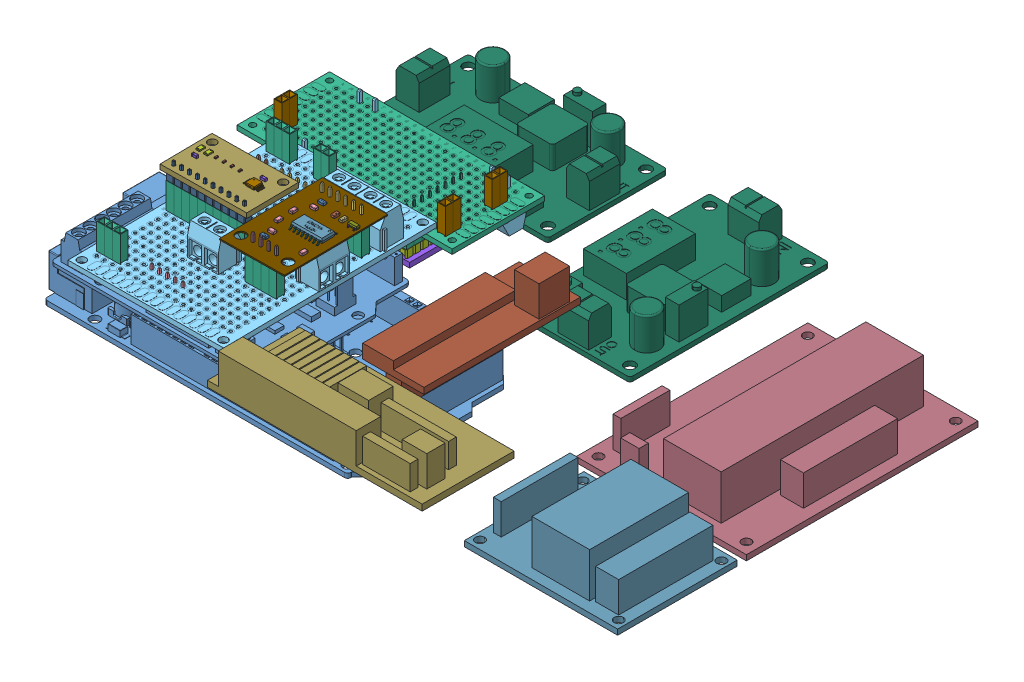
SolidWorks assembly ControlPCB, configuration Default. Lengths in mm.
Overall size (144.9 41.12 153.13).
136 component instances, 33 part files, 35 mates.
Components (placement in the parent):
- MEGA2560+MotorShield-1: MEGA2560+MotorShield [Default] at origin size (108.32 25.5 53.3)
- 1x2 Male Pin Header.step-1: 1x2 Male Pin Header.step [Default] at (-30.15 23.54 -23.8673) x (1 0 0) z (0 0 -1) size (5.08 13.54 2.5)
- 1x6 Male Pin Header.step-1: 1x6 Male Pin Header.step [Default] at (-9.8 23.54 -23.8673) x (-1 0 0) z (0 0 1) size (15.24 13.54 2.5)
- 1x5 Male Pin Header.step-1: 1x5 Male Pin Header.step [Default] at (-16.9 23.54 24.12) x (1 0 0) z (0 0 -1) size (12.71 13.54 2.5)
- ADCPCB-1: ADCPCB [Default] at (-8.2861 23.54 0.0047) x (0.011416 0 0.999935) z (0 1 0) size (70.2 51.25 24.04)
  - 5x7PCBBoard.stp-1: 5x7PCBBoard.stp [Default] at origin size (70.2 50.2 1.66)
  - FemalePinHeader2By1.stp-1: FemalePinHeader2By1.stp [Default] at (-29.21 -21.59 1.54) x (0 1 0) z (0 0 1) size (5.08 2.54 11.7)
    - Female Pin Header 1x.stp-1: Female Pin Header 1x.stp [Default] at origin size (2.54 2.54 11.7)
    - Female Pin Header 1x.stp-2: Female Pin Header 1x.stp [Default] at (2.54 0 0) size (2.54 2.54 11.7)
  - FemalePinHeader2By1.stp-2: FemalePinHeader2By1.stp [Default] at (-29.21 -6.35 1.54) x (0 1 0) z (0 0 1) size (5.08 2.54 11.7)
    - Female Pin Header 1x.stp-1: Female Pin Header 1x.stp [Default] at origin size (2.54 2.54 11.7)
    - Female Pin Header 1x.stp-2: Female Pin Header 1x.stp [Default] at (2.54 0 0) size (2.54 2.54 11.7)
  - FemalePinHeader2By1.stp-3: FemalePinHeader2By1.stp [Default] at (-29.21 -19.05 1.54) x (0 1 0) z (0 0 1) size (5.08 2.54 11.7)
    - Female Pin Header 1x.stp-1: Female Pin Header 1x.stp [Default] at origin size (2.54 2.54 11.7)
    - Female Pin Header 1x.stp-2: Female Pin Header 1x.stp [Default] at (2.54 0 0) size (2.54 2.54 11.7)
  - FemalePinHeader2By1.stp-4: FemalePinHeader2By1.stp [Default] at (26.67 -21.59 1.54) x (0 1 0) z (0 0 1) size (5.08 2.54 11.7)
    - Female Pin Header 1x.stp-1: Female Pin Header 1x.stp [Default] at origin size (2.54 2.54 11.7)
    - Female Pin Header 1x.stp-2: Female Pin Header 1x.stp [Default] at (2.54 0 0) size (2.54 2.54 11.7)
  - FemalePinHeader2By1.stp-5: FemalePinHeader2By1.stp [Default] at (26.67 -19.05 1.54) x (0 1 0) z (0 0 1) size (5.08 2.54 11.7)
    - Female Pin Header 1x.stp-1: Female Pin Header 1x.stp [Default] at origin size (2.54 2.54 11.7)
    - Female Pin Header 1x.stp-2: Female Pin Header 1x.stp [Default] at (2.54 0 0) size (2.54 2.54 11.7)
  - FemalePinHeader10By1.stp-1: FemalePinHeader10By1.stp [Default] at (3.81 1.27 1.54) x (0 -1 0) z (0 0 1) size (25.4 2.54 11.7)
    - Female Pin Header 1x.stp-1: Female Pin Header 1x.stp [Default] at origin size (2.54 2.54 11.7)
    - Female Pin Header 1x.stp-2: Female Pin Header 1x.stp [Default] at (2.54 0 0) size (2.54 2.54 11.7)
    - Female Pin Header 1x.stp-3: Female Pin Header 1x.stp [Default] at (5.08 0 0) size (2.54 2.54 11.7)
    - Female Pin Header 1x.stp-4: Female Pin Header 1x.stp [Default] at (7.62 0 0) size (2.54 2.54 11.7)
    - Female Pin Header 1x.stp-5: Female Pin Header 1x.stp [Default] at (10.16 0 0) size (2.54 2.54 11.7)
    - Female Pin Header 1x.stp-6: Female Pin Header 1x.stp [Default] at (12.7 0 0) size (2.54 2.54 11.7)
    - Female Pin Header 1x.stp-7: Female Pin Header 1x.stp [Default] at (15.24 0 0) size (2.54 2.54 11.7)
    - Female Pin Header 1x.stp-8: Female Pin Header 1x.stp [Default] at (17.78 0 0) size (2.54 2.54 11.7)
    - Female Pin Header 1x.stp-9: Female Pin Header 1x.stp [Default] at (20.32 0 0) size (2.54 2.54 11.7)
    - Female Pin Header 1x.stp-10: Female Pin Header 1x.stp [Default] at (22.86 0 0) size (2.54 2.54 11.7)
  - FemalePinHeader6By1.stp-1: FemalePinHeader6By1.stp [Default] at (-13.97 21.59 1.54) x (0 -1 0) z (0 0 1) size (15.24 2.54 11.7)
    - Female Pin Header 1x.stp-1: Female Pin Header 1x.stp [Default] at origin size (2.54 2.54 11.7)
    - Female Pin Header 1x.stp-2: Female Pin Header 1x.stp [Default] at (2.54 0 0) size (2.54 2.54 11.7)
    - Female Pin Header 1x.stp-3: Female Pin Header 1x.stp [Default] at (5.08 0 0) size (2.54 2.54 11.7)
    - Female Pin Header 1x.stp-4: Female Pin Header 1x.stp [Default] at (7.62 0 0) size (2.54 2.54 11.7)
    - Female Pin Header 1x.stp-5: Female Pin Header 1x.stp [Default] at (10.16 0 0) size (2.54 2.54 11.7)
    - Female Pin Header 1x.stp-6: Female Pin Header 1x.stp [Default] at (12.7 0 0) size (2.54 2.54 11.7)
  - FemalePinHeader4By1.stp-1: FemalePinHeader4By1.stp [Default] at (11.44 19.05 1.54) x (0 -1 0) z (0 0 1) size (10.16 2.54 11.7)
    - Female Pin Header 1x.stp-1: Female Pin Header 1x.stp [Default] at origin size (2.54 2.54 11.7)
    - Female Pin Header 1x.stp-2: Female Pin Header 1x.stp [Default] at (2.54 0 0) size (2.54 2.54 11.7)
    - Female Pin Header 1x.stp-3: Female Pin Header 1x.stp [Default] at (5.08 0 0) size (2.54 2.54 11.7)
    - Female Pin Header 1x.stp-4: Female Pin Header 1x.stp [Default] at (7.62 0 0) size (2.54 2.54 11.7)
  - ADS1115+PinHeader.step-1: ADS1115+PinHeader.step [Default] at (144.065 -99.14 12.63) x (-1 0 0) z (0 0 1) size (17.14 27.94 11.54)
    - R_0805_2012Metric.step-1: R_0805_2012Metric.step [Default] at (149.225 -80.01 1.65) size (2 1.2 0.45)
      - SOLID.step-1: SOLID.step [Default] at origin size (2 1.2 0.45)
    - R_0805_2012Metric.step-2: R_0805_2012Metric.step [Default] at (149.225 -77.47 1.65) size (2 1.2 0.45)
      - SOLID.step-1: SOLID.step [Default] at origin size (2 1.2 0.45)
    - C_0603_1608Metric.step-1: C_0603_1608Metric.step [Default] at (150.495 -96.52 1.65) x (0 1 0) z (0 0 1) size (1.6 0.8 0.8)
      - SOLID-0.step-1: SOLID-0.step [Default] at origin size (1.6 0.8 0.8)
    - TSSOP-10_3x3mm_P0.5mm.step-1: TSSOP-10_3x3mm_P0.5mm.step [Default] at (147.32 -96.52 1.65) x (0 -1 0) z (0 0 1) size (4.9 3 1)
      - SOLID-1.step-1: SOLID-1.step [Default] at origin size (4.9 3 1)
    - PinHeader_1x10_P2.54mm_Vertical.step-1: PinHeader_1x10_P2.54mm_Vertical.step [Default] at (140.335 -77.47 -0.05) x (-1 0 0) z (0 0 -1) size (2.54 25.4 11.54)
      - SOLID-2.step-1: SOLID-2.step [Default] at origin size (2.54 25.4 11.54)
    - C_0603_1608Metric.step-2: C_0603_1608Metric.step [Default] at (146.05 -78.74 1.65) x (0 1 0) z (0 0 1) size (1.6 0.8 0.8)
      - SOLID-0.step-1: SOLID-0.step [Default] at origin size (1.6 0.8 0.8)
    - R_0402_1005Metric.step-1: R_0402_1005Metric.step [Default] at (149.225 -85.09 1.65) x (-1 0 0) z (0 0 1) size (1 0.5 0.35)
      - SOLID-3.step-1: SOLID-3.step [Default] at origin size (1 0.5 0.35)
    - R_0402_1005Metric.step-2: R_0402_1005Metric.step [Default] at (149.225 -82.55 1.65) x (-1 0 0) z (0 0 1) size (1 0.5 0.35)
      - SOLID-3.step-1: SOLID-3.step [Default] at origin size (1 0.5 0.35)
    - R_0402_1005Metric.step-3: R_0402_1005Metric.step [Default] at (149.225 -87.63 1.65) size (1 0.5 0.35)
      - SOLID-3.step-1: SOLID-3.step [Default] at origin size (1 0.5 0.35)
    - R_0402_1005Metric.step-4: R_0402_1005Metric.step [Default] at (149.225 -90.17 1.65) x (-1 0 0) z (0 0 1) size (1 0.5 0.35)
      - SOLID-3.step-1: SOLID-3.step [Default] at origin size (1 0.5 0.35)
    - COMPOUND.step-1: COMPOUND.step [Default] at origin size (17.14 27.94 1.6)
  - 1x4 Male Pin Header.step-1: 1x4 Male Pin Header.step [Default] at (11.52 11.51 12.58) x (0 1 0) z (-1 0 0) size (10.17 13.54 2.5)
  - 1x6 Male Pin Header.step-1: 1x6 Male Pin Header.step [Default] at (-13.89 8.97 12.58) x (0 1 0) z (-1 0 0) size (15.24 13.54 2.5)
  - HX711.STEP-1: HX711.STEP [Default] at (-17.9207 5.1545 12.58) size (34 21 1.97)
    - HX711_SOP16_Valor predeterminado.STEP-1: HX711_SOP16_Valor predeterminado.STEP [Default] at (16.3915 14.4374 -9.5535) size (6.7 10 1.56)
      - base_HX711_Valor predeterminado.STEP-1: base_HX711_Valor predeterminado.STEP [Default] at (0.6189 -0.8581 10) size (4.4 10 1.52)
      - pino_HX711_Valor predeterminado.STEP-1: pino_HX711_Valor predeterminado.STEP [Default] at (-2.7311 3.5869 10.04) x (0 -1 0) z (-1 0 0) size (0.4 0.86 1.3)
      - pino_HX711_Valor predeterminado.STEP-2: pino_HX711_Valor predeterminado.STEP [Default] at (-2.7311 2.3169 10.04) x (0 -1 0) z (-1 0 0) size (0.4 0.86 1.3)
      - pino_HX711_Valor predeterminado.STEP-3: pino_HX711_Valor predeterminado.STEP [Default] at (-2.7311 1.0469 10.04) x (0 -1 0) z (-1 0 0) size (0.4 0.86 1.3)
      - pino_HX711_Valor predeterminado.STEP-4: pino_HX711_Valor predeterminado.STEP [Default] at (-2.7311 -0.2231 10.04) x (0 -1 0) z (-1 0 0) size (0.4 0.86 1.3)
      - pino_HX711_Valor predeterminado.STEP-5: pino_HX711_Valor predeterminado.STEP [Default] at (-2.7311 -1.4931 10.04) x (0 -1 0) z (-1 0 0) size (0.4 0.86 1.3)
      - pino_HX711_Valor predeterminado.STEP-6: pino_HX711_Valor predeterminado.STEP [Default] at (-2.7311 -2.7631 10.04) x (0 -1 0) z (-1 0 0) size (0.4 0.86 1.3)
      - pino_HX711_Valor predeterminado.STEP-7: pino_HX711_Valor predeterminado.STEP [Default] at (-2.7311 -4.0331 10.04) x (0 -1 0) z (-1 0 0) size (0.4 0.86 1.3)
      - pino_HX711_Valor predeterminado.STEP-8: pino_HX711_Valor predeterminado.STEP [Default] at (-2.7311 -5.3031 10.04) x (0 -1 0) z (-1 0 0) size (0.4 0.86 1.3)
      - pino_HX711_Valor predeterminado.STEP-9: pino_HX711_Valor predeterminado.STEP [Default] at (3.9689 3.5869 10.04) x (0 1 0) z (1 0 0) size (0.4 0.86 1.3)
      - pino_HX711_Valor predeterminado.STEP-10: pino_HX711_Valor predeterminado.STEP [Default] at (3.9689 2.3169 10.04) x (0 1 0) z (1 0 0) size (0.4 0.86 1.3)
      - pino_HX711_Valor predeterminado.STEP-11: pino_HX711_Valor predeterminado.STEP [Default] at (3.9689 1.0469 10.04) x (0 1 0) z (1 0 0) size (0.4 0.86 1.3)
      - pino_HX711_Valor predeterminado.STEP-12: pino_HX711_Valor predeterminado.STEP [Default] at (3.9689 -0.2231 10.04) x (0 1 0) z (1 0 0) size (0.4 0.86 1.3)
      - pino_HX711_Valor predeterminado.STEP-13: pino_HX711_Valor predeterminado.STEP [Default] at (3.9689 -1.4931 10.04) x (0 1 0) z (1 0 0) size (0.4 0.86 1.3)
      - pino_HX711_Valor predeterminado.STEP-14: pino_HX711_Valor predeterminado.STEP [Default] at (3.9689 -2.7631 10.04) x (0 1 0) z (1 0 0) size (0.4 0.86 1.3)
      - pino_HX711_Valor predeterminado.STEP-15: pino_HX711_Valor predeterminado.STEP [Default] at (3.9689 -4.0331 10.04) x (0 1 0) z (1 0 0) size (0.4 0.86 1.3)
      - pino_HX711_Valor predeterminado.STEP-16: pino_HX711_Valor predeterminado.STEP [Default] at (3.9689 -5.3031 10.04) x (0 1 0) z (1 0 0) size (0.4 0.86 1.3)
    - SOT23_Valor predeterminado.STEP-1: SOT23_Valor predeterminado.STEP [Default] at (9.1544 19.1355 -2.4535) x (-1 0 0) z (0 0 1) size (2.3 2.9 1.03)
      - TRANSISTOR_SOT23_Valor predeterminado.STEP-1: TRANSISTOR_SOT23_Valor predeterminado.STEP [Default] at (0.0204 0.1428 2.9) size (1.3 2.9 1)
      - PINO_SOT23_Valor predeterminado.STEP-1: PINO_SOT23_Valor predeterminado.STEP [Default] at (-1.1296 1.0928 2.94) x (0 -1 0) z (-1 0 0) size (0.4 0.61 0.65)
      - PINO_SOT23_Valor predeterminado.STEP-2: PINO_SOT23_Valor predeterminado.STEP [Default] at (-1.1296 -0.8072 2.94) x (0 -1 0) z (-1 0 0) size (0.4 0.61 0.65)
      - PINO_SOT23_Valor predeterminado.STEP-3: PINO_SOT23_Valor predeterminado.STEP [Default] at (1.1704 0.1428 2.94) x (0 1 0) z (1 0 0) size (0.4 0.61 0.65)
    - placa_Valor predeterminado.STEP-1: placa_Valor predeterminado.STEP [Default] at origin size (34 21 0.41)
    - RESISTOR_SMD_122_Valor predeterminado.STEP-1: RESISTOR_SMD_122_Valor predeterminado.STEP [Default] at (7.557 7.2289 0.4215) x (0 1 0) z (-1 0 0) size (2 0.82 1.27)
    - RESISTOR_SMD_122_Valor predeterminado.STEP-2: RESISTOR_SMD_122_Valor predeterminado.STEP [Default] at (26.4556 7.0756 0.4215) x (0 1 0) z (-1 0 0) size (2 0.82 1.27)
    - RESISTOR_SMD_822_Valor predeterminado.STEP-1: RESISTOR_SMD_822_Valor predeterminado.STEP [Default] at (8.9272 12.9039 0.4215) x (-1 0 0) z (0 -1 0) size (2 0.82 1.27)
    - RESISTOR_SMD_203_Valor predeterminado.STEP-1: RESISTOR_SMD_203_Valor predeterminado.STEP [Default] at (8.9446 15.4759 0.4215) x (-1 0 0) z (0 -1 0) size (2 0.82 1.27)
    - CAPACITOR_805_Valor predeterminado.STEP-1: CAPACITOR_805_Valor predeterminado.STEP [Default] at (14.517 4.7561 0.4215) x (1 0 0) z (0 1 0) size (2 0.8 1.27)
    - CAPACITOR_805_Valor predeterminado.STEP-2: CAPACITOR_805_Valor predeterminado.STEP [Default] at (24.8147 18.1011 0.4215) x (1 0 0) z (0 1 0) size (2 0.8 1.27)
    - CAPACITOR_805_Valor predeterminado.STEP-3: CAPACITOR_805_Valor predeterminado.STEP [Default] at (19.4533 4.8571 0.4215) x (1 0 0) z (0 1 0) size (2 0.8 1.27)
    - CAPACITOR_805_Valor predeterminado.STEP-4: CAPACITOR_805_Valor predeterminado.STEP [Default] at (23.7861 6.9684 0.4215) x (0 -1 0) z (1 0 0) size (2 0.8 1.27)
    - CAPACITOR_805_Valor predeterminado.STEP-5: CAPACITOR_805_Valor predeterminado.STEP [Default] at (10.279 7.2922 0.4215) x (0 -1 0) z (1 0 0) size (2 0.8 1.27)
  - 1x2 Male Pin Header.step-1: 1x2 Male Pin Header.step [Default] at (-29.29 -19.13 10.04) x (0 -1 0) z (-1 0 0) size (5.08 13.54 2.5) (hidden)
  - 1x2 Male Pin Header.step-2: 1x2 Male Pin Header.step [Default] at (-29.29 -3.89 10.04) x (0 -1 0) z (-1 0 0) size (5.08 13.54 2.5) (hidden)
  - 1x2 Male Pin Header.step-3: 1x2 Male Pin Header.step [Default] at (26.59 -16.59 10.04) x (0 -1 0) z (-1 0 0) size (5.08 13.54 2.5) (hidden)
  - 5mm2PTerminalBlock-1: 5mm2PTerminalBlock [Default] at (-25.19 24.09 1.54) x (0 -1 0) z (0 0 1) size (10.6 7.6 15)
  - 5mm2PTerminalBlock-2: 5mm2PTerminalBlock [Default] at (-25.19 13.89 1.54) x (0 -1 0) z (0 0 1) size (10.6 7.6 15)
  - 5mm2PTerminalBlock-3: 5mm2PTerminalBlock [Default] at (3.69 25.19 1.54) x (-1 0 0) z (0 0 1) size (10.6 7.6 15)
  - 5mm2PTerminalBlock-4: 5mm2PTerminalBlock [Default] at (15.04 -6.23 1.54) x (0 1 0) z (0 0 1) size (10.6 7.6 15)
- BLEShuntPCB-1: BLEShuntPCB [Default] at (-12.5947 21 -49.5125) x (-1 0 0) z (0 -1 0) size (73.24 30.62 25.87)
  - 3x7PerfBoard-1: 3x7PerfBoard [Default] at origin size (70.1 30.1 1.65)
  - 5mm2PTerminalBlock-1: 5mm2PTerminalBlock [Default] at (-19.17 15.03 1.55) x (-1 0 0) z (0 0 1) size (10.6 7.6 15)
  - FemalePinHeader8By1.stp-1: FemalePinHeader8By1.stp [Default] at (-16.51 6.35 1.55) x (0 -1 0) z (0 0 1) size (20.32 2.54 11.7)
    - Female Pin Header 1x.stp-1: Female Pin Header 1x.stp [Default] at origin size (2.54 2.54 11.7)
    - Female Pin Header 1x.stp-2: Female Pin Header 1x.stp [Default] at (2.54 0 0) size (2.54 2.54 11.7)
    - Female Pin Header 1x.stp-3: Female Pin Header 1x.stp [Default] at (5.08 0 0) size (2.54 2.54 11.7)
    - Female Pin Header 1x.stp-4: Female Pin Header 1x.stp [Default] at (7.62 0 0) size (2.54 2.54 11.7)
    - Female Pin Header 1x.stp-5: Female Pin Header 1x.stp [Default] at (10.16 0 0) size (2.54 2.54 11.7)
    - Female Pin Header 1x.stp-6: Female Pin Header 1x.stp [Default] at (12.7 0 0) size (2.54 2.54 11.7)
    - Female Pin Header 1x.stp-7: Female Pin Header 1x.stp [Default] at (15.24 0 0) size (2.54 2.54 11.7)
    - Female Pin Header 1x.stp-8: Female Pin Header 1x.stp [Default] at (17.78 0 0) size (2.54 2.54 11.7)
  - 1x8 Male Pin Header.step-1: 1x8 Male Pin Header.step [Default] at (-16.59 6.27 12.59) x (0 -1 0) z (1 0 0) size (20.32 13.54 2.5)
  - BLEFriend.stp-1: BLEFriend.stp [Default] at (-19.31 8.128 12.59) x (0 -1 0) z (0 0 1) size (21.35 31.87 4.78)
  - 5mm2PTerminalBlock-2: 5mm2PTerminalBlock [Default] at (24.01 15.03 1.55) x (-1 0 0) z (0 0 1) size (10.6 7.6 15)
  - 5mm2PTerminalBlock-5: 5mm2PTerminalBlock [Default] at (14.1 -15.03 1.55) size (10.6 7.6 15)
  - FemalePinHeader2By1-1: FemalePinHeader2By1 [Default] at (-29.21 -8.89 0) x (0 -1 0) z (0 0 -1) size (5.08 2.54 11.7)
  - FemalePinHeader2By1-2: FemalePinHeader2By1 [Default] at (-29.21 6.35 0) x (0 -1 0) z (0 0 -1) size (5.08 2.54 11.7)
  - FemalePinHeader2By1-3: FemalePinHeader2By1 [Default] at (26.67 -6.35 0) x (0 -1 0) z (0 0 -1) size (5.08 2.54 11.7)
  - ShuntResistor-1: ShuntResistor [Default<As Machined>] at (18.3281 0.2483 1.55) x (0.946299 -0.323291 0) z (-0.323291 -0.946299 0) size (35 9.71 20.4)
- RelayPCB-1: RelayPCB [Default] at (46.44 18.5 -16.8) x (0 0 -1) z (1 0 0) size (51 20.5 20)
- ThermistorPCB-1: ThermistorPCB [Default] at (53.61 18 26.48) x (0 0 -1) z (1 0 0) size (30 20 70)
- RelayPCB-2: RelayPCB [Default] at (109.78 0 -53.12) size (55.5 16.25 117.54)
  - 4-Port Relay-1: 4-Port Relay [Default] at origin size (55.5 16.25 75.54) (hidden)
  - 2-Port Relay-1: 2-Port Relay [Default] at (2.75 0 60.27) size (50 16.25 39) (hidden)
- LM2596-BuckConverter-1: LM2596-BuckConverter [Default] at (-16.99 0 -92.15) x (-1 0 0) z (0 1 0) size (65 39 13)
- LM2596-BuckConverter-2: LM2596-BuckConverter [Default] at (48.77 0 -79.15) x (0 0 -1) z (0 1 0) size (65 39 13)
Mates (geometry in assembly coordinates):
- Coincident1: coincident aligned: plane of MEGA2560+MotorShield-1 through (0 0 0) normal (0 0 1)
- Coincident2: coincident aligned: plane of MEGA2560+MotorShield-1 through (0 0 0) normal (0 1 0)
- Coincident3: coincident aligned: plane of MEGA2560+MotorShield-1 through (0 0 0) normal (1 0 0)
- Coincident4: coincident anti-aligned: plane of MEGA2560+MotorShield-1 through (-6.52 21 -22.6873) normal (0 1 0); plane of 1x2 Male Pin Header.step-1 through (-30.15 21 -23.8673) normal (0 -1 0)
- Coincident5: coincident anti-aligned: plane of MEGA2560+MotorShield-1 through (-30.47 13 -24.1873) normal (0 0 1); plane of 1x2 Male Pin Header.step-1 through (-30.47 13 -24.1873) normal (0 0 -1)
- Coincident6: coincident anti-aligned: plane of MEGA2560+MotorShield-1 through (-30.47 13 -23.6873) normal (1 0 0); plane of 1x2 Male Pin Header.step-1 through (-30.47 13 -24.1873) normal (-1 0 0)
- Coincident7: coincident anti-aligned: plane of MEGA2560+MotorShield-1 through (-6.52 21 -22.6873) normal (0 1 0); plane of 1x6 Male Pin Header.step-1 through (-22.5 21 -23.8673) normal (0 -1 0)
- Coincident8: coincident anti-aligned: plane of MEGA2560+MotorShield-1 through (-22.82 13 -24.1873) normal (0 0 1); plane of 1x6 Male Pin Header.step-1 through (-22.18 13 -24.1873) normal (0 0 -1)
- Coincident9: coincident anti-aligned: plane of MEGA2560+MotorShield-1 through (-22.82 13 -23.6873) normal (1 0 0); plane of 1x6 Male Pin Header.step-1 through (-22.82 13 -23.5473) normal (-1 0 0)
- Coincident10: coincident anti-aligned: plane of MEGA2560+MotorShield-1 through (2.78 21 22.8) normal (0 1 0); plane of 1x5 Male Pin Header.step-1 through (-16.9 21 24.12) normal (0 -1 0)
- Coincident11: coincident anti-aligned: plane of MEGA2560+MotorShield-1 through (-17.22 13 23.8) normal (0 0 1); plane of 1x5 Male Pin Header.step-1 through (-17.22 13 23.8) normal (0 0 -1)
- Coincident12: coincident anti-aligned: plane of MEGA2560+MotorShield-1 through (-17.22 13 24.3) normal (1 0 0); plane of 1x5 Male Pin Header.step-1 through (-17.22 13 23.8) normal (-1 0 0)
- Width1: width: cylinder of 1x2 Male Pin Header.step-1; plane of ADCPCB-1/5x7PCBBoard.stp-1 through (-30.47 13 -24.1873) normal (0 0 -1); cylinder of 1x2 Male Pin Header.step-1 through (-30.15 23.535 -23.8673) axis (0 -1 0) radius 0.45
- Coincident13: coincident anti-aligned: plane of 1x2 Male Pin Header.step-1 through (-30.15 23.54 -23.8673) normal (0 1 0); plane of ADCPCB-1/5x7PCBBoard.stp-1 through (-8.2861 23.54 0.0047) normal (0 -1 0)
- Width4: width: plane of 1x2 Male Pin Header.step-1 through (-30.47 13 -24.1873) normal (-1 0 0); plane of ADCPCB-1/5x7PCBBoard.stp-1 through (-29.83 13 -24.1873) normal (1 0 0); cylinder of 1x2 Male Pin Header.step-1 through (-30.15 23.535 -23.8673) axis (0 -1 0) radius 0.45
- Width5: width: plane of 1x5 Male Pin Header.step-1 through (-17.22 13 23.8) normal (-1 0 0); plane of ADCPCB-1/5x7PCBBoard.stp-1 through (-16.58 13 23.8) normal (1 0 0); cylinder of 1x5 Male Pin Header.step-1 through (-16.9 23.535 24.2346) axis (0 -1 0) radius 0.45
- Coincident17: coincident aligned: plane of MEGA2560+MotorShield-1 through (48.14 10 20.42) normal (1 0 0); plane of RelayPCB-1 through (48.14 10 7.7) normal (1 0 0)
- Coincident18: coincident anti-aligned: plane of MEGA2560+MotorShield-1 through (0 10 0) normal (0 1 0); plane of RelayPCB-1 through (46.44 10 -16.8) normal (0 -1 0)
- Coincident19: coincident aligned: plane of MEGA2560+MotorShield-1 through (43.06 10 -25.3) normal (0 0 -1); plane of RelayPCB-1 through (48.14 10 -25.3) normal (0 0 -1)
- Coincident20: coincident aligned: plane of MEGA2560+MotorShield-1 through (43.53 10 22.76) normal (1 0 0); plane of ThermistorPCB-1 through (43.53 10 25.3) normal (1 0 0)
- Coincident21: coincident aligned: plane of MEGA2560+MotorShield-1 through (23.21 10 25.3) normal (0 0 1); plane of ThermistorPCB-1 through (43.53 10 25.3) normal (0 0 1)
- Coincident22: coincident anti-aligned: plane of MEGA2560+MotorShield-1 through (0 10 0) normal (0 1 0); plane of ThermistorPCB-1 through (53.61 10 26.48) normal (0 -1 0)
- Coincident23: coincident aligned: plane of MEGA2560+MotorShield-1 through (0 0 0) normal (0 -1 0); plane of RelayPCB-2/2-Port Relay-1 through (112.53 0 7.15) normal (0 -1 0)
- Coincident24: coincident aligned: plane of MEGA2560+MotorShield-1 through (-49.49 1.5 26.65) normal (0 0 1); plane of RelayPCB-2/2-Port Relay-1 through (137.53 1.75 26.65) normal (0 0 1)
- Distance1: distance = 30 mm anti-aligned: plane of RelayPCB-2/4-Port Relay-1 through (82.03 1.75 -90.89) normal (-1 0 0); plane of MEGA2560+MotorShield-1 through (52.03 1.5 -11.41) normal (1 0 0)
- Coincident26: coincident aligned: plane of MEGA2560+MotorShield-1 through (0 0 0) normal (0 -1 0); plane of LM2596-BuckConverter-1 through (-16.99 0 -92.15) normal (0 -1 0)
- Coincident27: coincident aligned: plane of MEGA2560+MotorShield-1 through (-49.49 1.5 -26.65) normal (-1 0 0); plane of LM2596-BuckConverter-1 through (-49.49 1.5 -111.65) normal (-1 0 0)
- Coincident30: coincident aligned: plane of MEGA2560+MotorShield-1 through (0 0 0) normal (0 -1 0); plane of LM2596-BuckConverter-2 through (48.77 0 -79.15) normal (0 -1 0)
- Symmetric1: symmetric aligned: plane of RelayPCB-2/4-Port Relay-1 through (82.03 1.75 -90.89) normal (-1 0 0); plane of LM2596-BuckConverter-1 through (15.51 1.5 -111.65) normal (1 0 0); plane of LM2596-BuckConverter-2 through (48.77 0 -79.15) normal (-1 0 0)
- Distance2: distance = 20 mm anti-aligned: plane of LM2596-BuckConverter-2 through (68.27 1.5 -46.65) normal (0 0 1); plane of MEGA2560+MotorShield-1 through (-49.49 1.5 -26.65) normal (0 0 -1)
- Coincident37: coincident aligned: plane of LM2596-BuckConverter-1 through (15.51 1.5 -111.65) normal (0 0 -1); plane of LM2596-BuckConverter-2 through (68.27 1.5 -111.65) normal (0 0 -1)
- Parallel3: parallel aligned: plane of ADCPCB-1/5x7PCBBoard.stp-1 through (-8.2861 25.08 0.0047) normal (0 1 0); plane of BLEShuntPCB-1/3x7PerfBoard-1 through (-12.5947 21 -49.5125) normal (0 1 0)
- Coincident41: coincident aligned: plane of BLEShuntPCB-1/3x7PerfBoard-1 through (-47.6447 21 -64.5625) normal (-1 0 0); plane of MEGA2560+MotorShield-1 through (-47.6447 12 25.0622) normal (-1 0 0)
- Coincident42: coincident aligned: plane of MEGA2560+MotorShield-1 through (-6.52 21 -22.6873) normal (0 1 0); plane of BLEShuntPCB-1/3x7PerfBoard-1 through (-12.5947 21 -49.5125) normal (0 1 0)
- Distance3: distance = 38 mm aligned: plane of BLEShuntPCB-1/3x7PerfBoard-1 through (22.4553 21 -64.5625) normal (0 0 -1); plane of MEGA2560+MotorShield-1 through (-46.2695 12 -26.5625) normal (0 0 -1)
